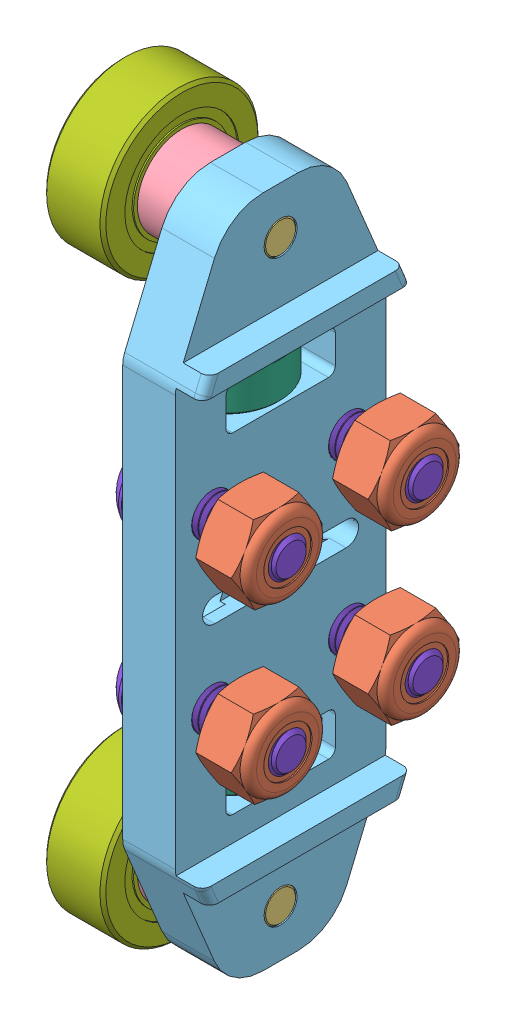
SolidWorks assembly Bearing Block, configuration Default. Lengths in mm.
Overall size (31.06 89.43 29.43).
19 component instances, 8 part files, 0 mates.
Components (placement in the parent):
- Sliding Elevator Bearing Block Kit.step-1: Sliding Elevator Bearing Block Kit.step [Default] at (-2.279 1755.626 148.4607) x (0 -0.999847 -0.017493) z (-1 0 0) size (88.96 27.87 31.06)
  - .25diameter_1.75inSteelDowel_SLIDE-002.step-1: .25diameter_1.75inSteelDowel_SLIDE-002.step [Default] at (428.3334 525.2741 706.1052) x (0.999847 0.017493 0) z (0 0 1) size (44.45 6.35 6.35)
  - 10-32 Locknut 2623.step-1: 10-32 Locknut 2623.step [Default] at (418.0305 533.3501 696.4532) x (1 0 0) z (0 1 0) size (9.53 5.96 11)
  - Bearing Block Shoulder Bolt - SLIDE-004.step-1: Bearing Block Shoulder Bolt - SLIDE-004.step [Default] at (393.4137 524.6631 723.447) x (0.999978 0.006628 0) z (0 0 1) size (9.53 9.53 21.53)
  - Bearing Block Shoulder Bolt Spacer - SLIDE-003.step-1: Bearing Block Shoulder Bolt Spacer - SLIDE-003.step [Default] at (209.8469 202.8854 705.9782) x (0.999977 0.006804 0) z (0 0 1) size (10.72 10.72 5.56)
  - Sliding Bearing Block Plate - SLIDE-001.step-1: Sliding Bearing Block Plate - SLIDE-001.step [Default] at (417.8216 -325.94 699.6282) x (0.999847 0.017493 0) z (0 0 1) size (81.28 25.4 9.54)
  - TTB-0027_.50OD_.25ID_.188WD.step-1: TTB-0027_.50OD_.25ID_.188WD.step [Default] at (448.2757 525.623 706.1052) x (0 0 -1) z (0.999847 0.017493 0) size (12.7 12.7 4.76)
  - TTB-0038_75OD_25ID_28WD.step-1: TTB-0038_75OD_25ID_28WD.step [Default] at (463.253 525.885 715.1127) size (19.05 19.05 7.14)
  - Bearing Block Shoulder Bolt - SLIDE-004.step-2: Bearing Block Shoulder Bolt - SLIDE-004.step [Default] at (463.253 525.885 723.447) size (9.53 9.53 21.53)
  - TTB-0027_.50OD_.25ID_.188WD.step-2: TTB-0027_.50OD_.25ID_.188WD.step [Default] at (408.3911 524.9252 706.1052) x (0 0 -1) z (0.999847 0.017493 0) size (12.7 12.7 4.76)
  - Bearing Block Shoulder Bolt Spacer - SLIDE-003.step-2: Bearing Block Shoulder Bolt Spacer - SLIDE-003.step [Default] at (277.5012 205.3636 705.9782) size (10.72 10.72 5.56)
  - TTB-0038_75OD_25ID_28WD.step-2: TTB-0038_75OD_25ID_28WD.step [Default] at (393.4137 524.6631 715.1127) x (0.999973 0.007362 0) z (0 0 1) size (19.05 19.05 7.14)
  - .625 Long 10-32 Button Head Screw.step-1: .625 Long 10-32 Button Head Screw.step [Default] at (438.3474 533.7055 699.3234) x (0.999998 0.002032 0) z (0 0 1) size (9.17 9.17 18.44)
  - .625 Long 10-32 Button Head Screw.step-2: .625 Long 10-32 Button Head Screw.step [Default] at (438.6362 517.1981 699.3234) x (1 -0.000148 0) z (0 0 1) size (9.17 9.17 18.44)
  - .625 Long 10-32 Button Head Screw.step-3: .625 Long 10-32 Button Head Screw.step [Default] at (418.3193 516.8426 699.3234) x (0.999999 0.001159 0) z (0 0 1) size (9.17 9.17 18.44)
  - .625 Long 10-32 Button Head Screw.step-4: .625 Long 10-32 Button Head Screw.step [Default] at (418.0305 533.3501 699.3234) x (0.999983 0.005862 0) z (0 0 1) size (9.17 9.17 18.44)
  - 10-32 Locknut 2623.step-2: 10-32 Locknut 2623.step [Default] at (438.3474 533.7055 696.4532) x (0.999999 0.001134 0) z (-0.001134 0.999999 0) size (9.53 5.96 11)
  - 10-32 Locknut 2623.step-3: 10-32 Locknut 2623.step [Default] at (438.6362 517.1981 696.4532) x (1 0.000493 0) z (-0.000493 1 0) size (9.53 5.96 11)
  - 10-32 Locknut 2623.step-4: 10-32 Locknut 2623.step [Default] at (418.3193 516.8426 696.4532) x (0.999999 0.001452 0) z (-0.001452 0.999999 0) size (9.53 5.96 11)
